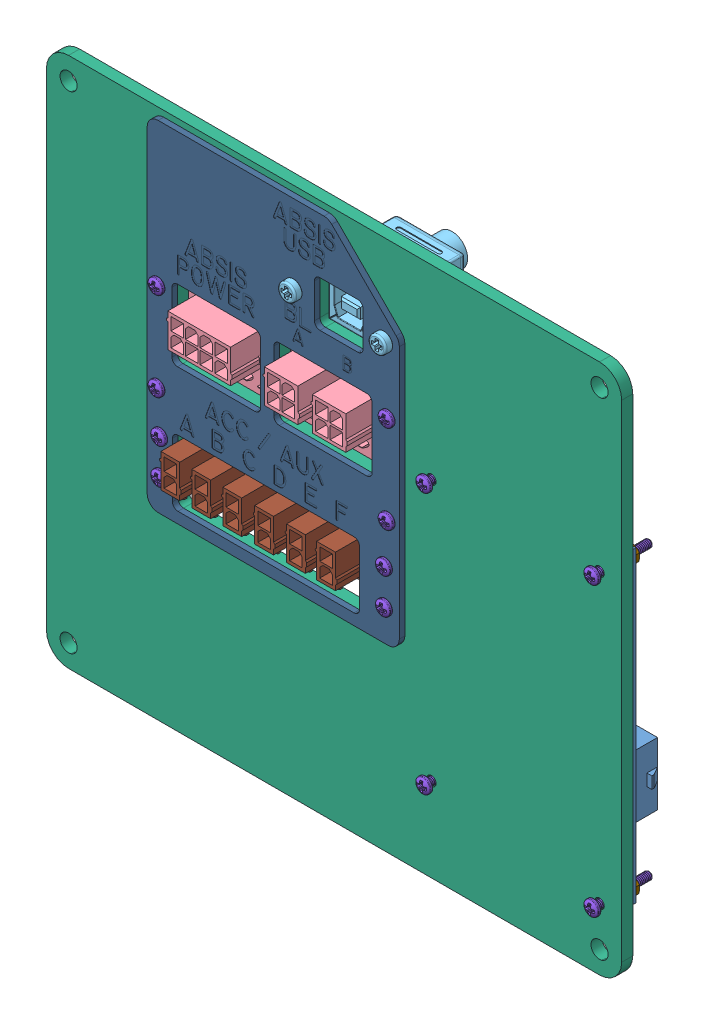
SolidWorks assembly Right Console Bulkhead Interconnect Panel, configuration Default. Lengths in mm.
Overall size (165.1 152.4 37.41).
47 component instances, 11 part files, 24 mates.
Components (placement in the parent):
- ABSIS_hid_bus_master_pcb-1: ABSIS_hid_bus_master_pcb [Default] at (-289.2033 2614.9961 -5883.3904) x (0 -1 0) z (0 0 -1) size (90.8 53.34 16.58)
  - ABSIS_hid_bus_master_pcb-1: ABSIS_hid_bus_master_pcb [Default] at (-243.5501 4.8834 76.9629) size (90.8 53.34 16.58)
  - HEADER, PIN, .1 SPACING-1: HEADER, PIN, .1 SPACING [1x12] at (-216.2801 51.8534 85.1199) x (-1 0 0) z (0 -1 0) size (30.48 11.54 2.54)
  - DEV-12640 - ARDUINO PRO MICRO, 5V, 16 MHz, SPARKFUN-1: DEV-12640 - ARDUINO PRO MICRO, 5V, 16 MHz, SPARKFUN [Default] at (-217.5501 37.8834 85.1199) x (1 0 0) z (0 -1 0) size (34.59 4.25 17.78)
  - HEADER, PIN, .1 SPACING-2: HEADER, PIN, .1 SPACING [1x12] at (-216.2801 36.6134 85.1199) x (-1 0 0) z (0 -1 0) size (30.48 11.54 2.54)
- ABSIS_Bulkhead_Connector-1: ABSIS_Bulkhead_Connector [Default] at (-525.8617 2925.8262 -5961.9533) x (1 0 0) z (0 0 1) size (76.2 35.56 27.3)
- 1581-01C - CABLE, USB 2.0, TYPE B FEMALE TO MICRO B MALE, 1 FT-1: 1581-01C - CABLE, USB 2.0, TYPE B FEMALE TO MICRO B MALE, 1 FT [USB TYPE B FEMALE] at (-369.8767 2883.2962 -6284.3783) x (-1 -0.000084 0) z (0 0 1) size (33.5 14.04 34.59)
- Right Console Bulkhead Connector Panel^OH5A1-1 - ASSY, RIGHT CONSOLE-1: Right Console Bulkhead Connector Panel^OH5A1-1 - ASSY, RIGHT CONSOLE [Default] at (-0.0817 1.6812 -5954.0033) x (-1 0 0) z (0 0 -1) size (165.1 152.4 3.17)
- 1581-01C - CABLE, USB 2.0, TYPE B FEMALE TO MICRO B MALE, 1 FT-2: 1581-01C - CABLE, USB 2.0, TYPE B FEMALE TO MICRO B MALE, 1 FT [USB TYPE B MICRO MALE] at (-334.7067 2858.208 -5971.2853) x (1 0 0) z (0 1 0) size (10.7 7.58 34.44)
- 94639A187 - SPACER, 2 X .250 OD X .125 L, NYL-1: 94639A187 - SPACER, 2 X .250 OD X .125 L, NYL [94639A187] at (-296.6267 2855.3712 -5958.7658) x (0.961477 0.274887 0) z (0 0 1) size (6.35 6.35 3.17)
- 91249A060 - PHS, 2-56 X .625, 18-8, BLACK OXIDE-2: 91249A060 - PHS, 2-56 X .625, 18-8, BLACK OXIDE [91249A060] at (-296.6267 2855.3712 -5968.2908) x (1 0 0) z (0 0 1) size (4.24 4.24 17.48)
- 95130A105 - NUT, 2-56, NARROW, BRASS-1: 95130A105 - NUT, 2-56, NARROW, BRASS [95130A105] at (-296.6267 2855.3712 -5962.747) x (0.996294 -0.086016 0) z (-0.086016 -0.996294 0) size (3.97 1.94 4.58)
- 95130A105 - NUT, 2-56, NARROW, BRASS-2: 95130A105 - NUT, 2-56, NARROW, BRASS [95130A105] at (-355.6817 2839.4662 -5962.747) x (0.996294 -0.086016 0) z (-0.086016 -0.996294 0) size (3.97 1.94 4.58)
- 95130A105 - NUT, 2-56, NARROW, BRASS-3: 95130A105 - NUT, 2-56, NARROW, BRASS [95130A105] at (-421.7217 2839.4662 -5962.747) x (0.996294 -0.086016 0) z (-0.086016 -0.996294 0) size (3.97 1.94 4.58)
- 95130A105 - NUT, 2-56, NARROW, BRASS-4: 95130A105 - NUT, 2-56, NARROW, BRASS [95130A105] at (-355.6817 2864.8662 -5962.747) x (0.996294 -0.086016 0) z (-0.086016 -0.996294 0) size (3.97 1.94 4.58)
- 95130A105 - NUT, 2-56, NARROW, BRASS-5: 95130A105 - NUT, 2-56, NARROW, BRASS [95130A105] at (-421.7217 2864.8662 -5962.747) x (0.996294 -0.086016 0) z (-0.086016 -0.996294 0) size (3.97 1.94 4.58)
- 95130A105 - NUT, 2-56, NARROW, BRASS-6: 95130A105 - NUT, 2-56, NARROW, BRASS [95130A105] at (-344.8867 2779.1712 -5962.747) x (0.996294 -0.086016 0) z (-0.086016 -0.996294 0) size (3.97 1.94 4.58)
- 95130A105 - NUT, 2-56, NARROW, BRASS-7: 95130A105 - NUT, 2-56, NARROW, BRASS [95130A105] at (-296.6267 2772.8212 -5962.747) x (0.996294 -0.086016 0) z (-0.086016 -0.996294 0) size (3.97 1.94 4.58)
- 95130A105 - NUT, 2-56, NARROW, BRASS-8: 95130A105 - NUT, 2-56, NARROW, BRASS [95130A105] at (-344.8867 2854.1012 -5962.747) x (0.996294 -0.086016 0) z (-0.086016 -0.996294 0) size (3.97 1.94 4.58)
- 91249A060 - PHS, 2-56 X .625, 18-8, BLACK OXIDE-3: 91249A060 - PHS, 2-56 X .625, 18-8, BLACK OXIDE [91249A060] at (-355.6817 2839.4662 -5968.2908) x (1 0 0) z (0 0 1) size (4.24 4.24 17.48)
- 91249A060 - PHS, 2-56 X .625, 18-8, BLACK OXIDE-4: 91249A060 - PHS, 2-56 X .625, 18-8, BLACK OXIDE [91249A060] at (-421.7217 2839.4662 -5968.2908) x (1 0 0) z (0 0 1) size (4.24 4.24 17.48)
- 91249A060 - PHS, 2-56 X .625, 18-8, BLACK OXIDE-5: 91249A060 - PHS, 2-56 X .625, 18-8, BLACK OXIDE [91249A060] at (-355.6817 2864.8662 -5968.2908) x (1 0 0) z (0 0 1) size (4.24 4.24 17.48)
- 91249A060 - PHS, 2-56 X .625, 18-8, BLACK OXIDE-6: 91249A060 - PHS, 2-56 X .625, 18-8, BLACK OXIDE [91249A060] at (-421.7217 2864.8662 -5968.2908) x (1 0 0) z (0 0 1) size (4.24 4.24 17.48)
- 91249A060 - PHS, 2-56 X .625, 18-8, BLACK OXIDE-7: 91249A060 - PHS, 2-56 X .625, 18-8, BLACK OXIDE [91249A060] at (-344.8867 2779.1712 -5968.2908) x (1 0 0) z (0 0 1) size (4.24 4.24 17.48)
- 91249A060 - PHS, 2-56 X .625, 18-8, BLACK OXIDE-8: 91249A060 - PHS, 2-56 X .625, 18-8, BLACK OXIDE [91249A060] at (-296.6267 2772.8212 -5968.2908) x (1 0 0) z (0 0 1) size (4.24 4.24 17.48)
- 91249A060 - PHS, 2-56 X .625, 18-8, BLACK OXIDE-9: 91249A060 - PHS, 2-56 X .625, 18-8, BLACK OXIDE [91249A060] at (-344.8867 2854.1012 -5968.2908) x (1 0 0) z (0 0 1) size (4.24 4.24 17.48)
- 94639A187 - SPACER, 2 X .250 OD X .125 L, NYL-2: 94639A187 - SPACER, 2 X .250 OD X .125 L, NYL [94639A187] at (-355.6817 2839.4662 -5958.7658) x (0.961477 0.274887 0) z (0 0 1) size (6.35 6.35 3.17)
- 94639A187 - SPACER, 2 X .250 OD X .125 L, NYL-3: 94639A187 - SPACER, 2 X .250 OD X .125 L, NYL [94639A187] at (-421.7217 2839.4662 -5958.7658) x (0.961477 0.274887 0) z (0 0 1) size (6.35 6.35 3.17)
- 94639A187 - SPACER, 2 X .250 OD X .125 L, NYL-4: 94639A187 - SPACER, 2 X .250 OD X .125 L, NYL [94639A187] at (-355.6817 2864.8662 -5958.7658) x (0.961477 0.274887 0) z (0 0 1) size (6.35 6.35 3.17)
- 94639A187 - SPACER, 2 X .250 OD X .125 L, NYL-5: 94639A187 - SPACER, 2 X .250 OD X .125 L, NYL [94639A187] at (-421.7217 2864.8662 -5958.7658) x (0.961477 0.274887 0) z (0 0 1) size (6.35 6.35 3.17)
- 94639A187 - SPACER, 2 X .250 OD X .125 L, NYL-6: 94639A187 - SPACER, 2 X .250 OD X .125 L, NYL [94639A187] at (-344.8867 2779.1712 -5958.7658) x (0.961477 0.274887 0) z (0 0 1) size (6.35 6.35 3.17)
- 94639A187 - SPACER, 2 X .250 OD X .125 L, NYL-7: 94639A187 - SPACER, 2 X .250 OD X .125 L, NYL [94639A187] at (-296.6267 2772.8212 -5958.7658) x (0.961477 0.274887 0) z (0 0 1) size (6.35 6.35 3.17)
- 94639A187 - SPACER, 2 X .250 OD X .125 L, NYL-8: 94639A187 - SPACER, 2 X .250 OD X .125 L, NYL [94639A187] at (-344.8867 2854.1012 -5958.7658) x (0.961477 0.274887 0) z (0 0 1) size (6.35 6.35 3.17)
- Right Console Bulkhead Interconnect Panel Legend Plate-1: Right Console Bulkhead Interconnect Panel Legend Plate [Default] at (0 0 -5954.0033) x (1 0 0) z (0 0 1) size (72.39 97.5 1.59)
- ABSIS_AUX_Bulkhead_Connector-1: ABSIS_AUX_Bulkhead_Connector [Default] at (-525.0997 2888.6787 -5961.9533) x (1 0 0) z (0 0 1) size (74.68 20.32 27.3)
- 94639A187 - SPACER, 2 X .250 OD X .125 L, NYL-9: 94639A187 - SPACER, 2 X .250 OD X .125 L, NYL [94639A187] at (-356.4437 2817.5587 -5958.7658) x (0.961477 0.274887 0) z (0 0 1) size (6.35 6.35 3.17)
- 94639A187 - SPACER, 2 X .250 OD X .125 L, NYL-10: 94639A187 - SPACER, 2 X .250 OD X .125 L, NYL [94639A187] at (-356.4437 2827.7187 -5958.7658) x (0.961477 0.274887 0) z (0 0 1) size (6.35 6.35 3.17)
- 94639A187 - SPACER, 2 X .250 OD X .125 L, NYL-11: 94639A187 - SPACER, 2 X .250 OD X .125 L, NYL [94639A187] at (-420.9597 2817.5587 -5958.7658) x (0.961477 0.274887 0) z (0 0 1) size (6.35 6.35 3.17)
- 94639A187 - SPACER, 2 X .250 OD X .125 L, NYL-12: 94639A187 - SPACER, 2 X .250 OD X .125 L, NYL [94639A187] at (-420.9597 2827.7187 -5958.7658) x (0.961477 0.274887 0) z (0 0 1) size (6.35 6.35 3.17)
- 91249A060 - PHS, 2-56 X .625, 18-8, BLACK OXIDE-10: 91249A060 - PHS, 2-56 X .625, 18-8, BLACK OXIDE [91249A060] at (-356.4437 2817.5587 -5968.2908) x (1 0 0) z (0 0 1) size (4.24 4.24 17.48)
- 91249A060 - PHS, 2-56 X .625, 18-8, BLACK OXIDE-11: 91249A060 - PHS, 2-56 X .625, 18-8, BLACK OXIDE [91249A060] at (-356.4437 2827.7187 -5968.2908) x (1 0 0) z (0 0 1) size (4.24 4.24 17.48)
- 91249A060 - PHS, 2-56 X .625, 18-8, BLACK OXIDE-12: 91249A060 - PHS, 2-56 X .625, 18-8, BLACK OXIDE [91249A060] at (-420.9597 2817.5587 -5968.2908) x (1 0 0) z (0 0 1) size (4.24 4.24 17.48)
- 91249A060 - PHS, 2-56 X .625, 18-8, BLACK OXIDE-13: 91249A060 - PHS, 2-56 X .625, 18-8, BLACK OXIDE [91249A060] at (-420.9597 2827.7187 -5968.2908) x (1 0 0) z (0 0 1) size (4.24 4.24 17.48)
- 95130A105 - NUT, 2-56, NARROW, BRASS-9: 95130A105 - NUT, 2-56, NARROW, BRASS [95130A105] at (-356.4437 2817.5587 -5962.747) x (0.996294 -0.086016 0) z (-0.086016 -0.996294 0) size (3.97 1.94 4.58)
- 95130A105 - NUT, 2-56, NARROW, BRASS-10: 95130A105 - NUT, 2-56, NARROW, BRASS [95130A105] at (-356.4437 2827.7187 -5962.747) x (0.996294 -0.086016 0) z (-0.086016 -0.996294 0) size (3.97 1.94 4.58)
- 95130A105 - NUT, 2-56, NARROW, BRASS-11: 95130A105 - NUT, 2-56, NARROW, BRASS [95130A105] at (-420.9597 2817.5587 -5962.747) x (0.996294 -0.086016 0) z (-0.086016 -0.996294 0) size (3.97 1.94 4.58)
- 95130A105 - NUT, 2-56, NARROW, BRASS-12: 95130A105 - NUT, 2-56, NARROW, BRASS [95130A105] at (-420.9597 2827.7187 -5962.747) x (0.996294 -0.086016 0) z (-0.086016 -0.996294 0) size (3.97 1.94 4.58)
Mates (geometry in assembly coordinates):
- Distance5: distance = 3.175 mm anti-aligned: plane of ABSIS_hid_bus_master_pcb-1/ABSIS_hid_bus_master_pcb-1 through (-320.5698 2813.9836 -5960.3533) normal (0 0 1); plane of Right Console Bulkhead Connector Panel^OH5A1-1 - ASSY, RIGHT CONSOLE-1 through (-0.0817 1.6812 -5957.1783) normal (0 0 -1)
- Distance6: distance = 6.35 mm: cylinder of ABSIS_hid_bus_master_pcb-1/ABSIS_hid_bus_master_pcb-1 through (-296.6267 2772.8212 -5959.5533) axis (0 0 -1) radius 1.524; plane of Right Console Bulkhead Connector Panel^OH5A1-1 - ASSY, RIGHT CONSOLE-1 through (-290.2767 2907.4412 -5957.1783) normal (1 0 0)
- Distance7: distance = 6.35 mm: plane of ABSIS_hid_bus_master_pcb-1/ABSIS_hid_bus_master_pcb-1 through (-297.8967 2767.7412 -5960.3533) normal (0 -1 0); cylinder of Right Console Bulkhead Connector Panel^OH5A1-1 - ASSY, RIGHT CONSOLE-1 through (-296.6267 2761.3912 -5957.1783) axis (0 0 -1) radius 2.4574
- Parallel19: parallel aligned: plane of ABSIS_hid_bus_master_pcb-1/ABSIS_hid_bus_master_pcb-1 through (-294.0867 2858.5462 -5960.3533) normal (1 0 0); plane of Right Console Bulkhead Connector Panel^OH5A1-1 - ASSY, RIGHT CONSOLE-1 through (-290.2767 2907.4412 -5957.1783) normal (1 0 0)
- Distance8: distance = 12.7 mm anti-aligned: plane of 1581-01C - CABLE, USB 2.0, TYPE B FEMALE TO MICRO B MALE, 1 FT-1 through (-360.1267 2876.2962 -5979.5783) normal (1 0 0); plane of ABSIS_hid_bus_master_pcb-1/ABSIS_hid_bus_master_pcb-1 through (-347.4267 2772.8212 -5960.3533) normal (-1 0 0)
- Parallel20: parallel aligned: plane of ABSIS_hid_bus_master_pcb-1/DEV-12640 - ARDUINO PRO MICRO, 5V, 16 MHz, SPARKFUN-1 through (-331.4567 2832.2962 -5972.4603) normal (0 0 -1); plane of 1581-01C - CABLE, USB 2.0, TYPE B FEMALE TO MICRO B MALE, 1 FT-2 through (-337.6867 2849.666 -5972.1703) normal (0 0 -1)
- Symmetric1: symmetric aligned: plane of ABSIS_hid_bus_master_pcb-1/DEV-12640 - ARDUINO PRO MICRO, 5V, 16 MHz, SPARKFUN-1 through (-338.4067 2832.2962 -5972.0103) normal (-1 0 0); plane of 1581-01C - CABLE, USB 2.0, TYPE B FEMALE TO MICRO B MALE, 1 FT-2 through (-331.0067 2832.2962 -5971.1931) normal (1 0 0); plane of ABSIS_hid_bus_master_pcb-1/DEV-12640 - ARDUINO PRO MICRO, 5V, 16 MHz, SPARKFUN-1 through (-334.7067 2858.208 -5971.2853) normal (1 0 0)
- Symmetric2: symmetric aligned: plane of ABSIS_hid_bus_master_pcb-1/DEV-12640 - ARDUINO PRO MICRO, 5V, 16 MHz, SPARKFUN-1 through (-331.4567 2832.2962 -5972.4603) normal (0 0 -1); plane of 1581-01C - CABLE, USB 2.0, TYPE B FEMALE TO MICRO B MALE, 1 FT-2 through (-334.7067 2832.2962 -5970.1103) normal (0 0 1); plane of ABSIS_hid_bus_master_pcb-1/DEV-12640 - ARDUINO PRO MICRO, 5V, 16 MHz, SPARKFUN-1 through (-334.7067 2858.208 -5971.2853) normal (0 0 -1)
- Coincident197: coincident: line of ABSIS_hid_bus_master_pcb-1/DEV-12640 - ARDUINO PRO MICRO, 5V, 16 MHz, SPARKFUN-1 through (-331.9317 2836.2962 -5972.6274) axis (-1 0 0); plane of 1581-01C - CABLE, USB 2.0, TYPE B FEMALE TO MICRO B MALE, 1 FT-2 through (-332.1317 2836.2962 -5972.6753) normal (0 1 0)
- Distance9: distance = 9.525 mm anti-aligned: plane of ABSIS_Bulkhead_Connector-1 through (-387.9565 2818.735 -5967.73) normal (0 0 1); plane of Right Console Bulkhead Connector Panel^OH5A1-1 - ASSY, RIGHT CONSOLE-1 through (0 0 -5958.205) normal (0 0 -1)
- Distance10: distance = 6.35 mm anti-aligned: plane of ABSIS_Bulkhead_Connector-1 through (-426.8017 2869.9462 -5961.9533) normal (0 1 0); plane of 1581-01C - CABLE, USB 2.0, TYPE B FEMALE TO MICRO B MALE, 1 FT-1 through (-379.6267 2876.2962 -5979.5783) normal (0 -1 0)
- Coincident195: coincident anti-aligned: plane of Right Console Bulkhead Connector Panel^OH5A1-1 - ASSY, RIGHT CONSOLE-1 through (-0.0817 1.6812 -5957.1783) normal (0 0 -1); plane of 1581-01C - CABLE, USB 2.0, TYPE B FEMALE TO MICRO B MALE, 1 FT-1 through (-369.8767 2883.2962 -5957.1783) normal (0 0 1)
- Distance11: distance = 3.175 mm anti-aligned: plane of ABSIS_Bulkhead_Connector-1 through (-388.7017 2852.1662 -5960.3533) normal (0 0 1); plane of Right Console Bulkhead Connector Panel^OH5A1-1 - ASSY, RIGHT CONSOLE-1 through (-0.0817 1.6812 -5957.1783) normal (0 0 -1)
- Distance12: distance = 3.175 mm anti-aligned: plane of ABSIS_hid_bus_master_pcb-1/ABSIS_hid_bus_master_pcb-1 through (-347.4267 2772.8212 -5960.3533) normal (-1 0 0); plane of ABSIS_Bulkhead_Connector-1 through (-350.6017 2869.9462 -5961.9533) normal (1 0 0)
- Concentric1: concentric aligned: cylinder of Right Console Bulkhead Connector Panel^OH5A1-1 - ASSY, RIGHT CONSOLE-1 through (-296.6267 2855.3712 -5957.1783) axis (0 0 -1) radius 1.3526; cylinder of 94639A187 - SPACER, 2 X .250 OD X .125 L, NYL-1 through (-296.6267 2855.3712 -5957.1783) axis (0 0 -1) radius 3.175
- Coincident198: coincident anti-aligned: plane of Right Console Bulkhead Connector Panel^OH5A1-1 - ASSY, RIGHT CONSOLE-1 through (-0.0817 1.6812 -5957.1783) normal (0 0 -1); plane of 94639A187 - SPACER, 2 X .250 OD X .125 L, NYL-1 through (-296.6267 2855.3712 -5957.1783) normal (0 0 1)
- Concentric3: concentric aligned: cylinder of Right Console Bulkhead Connector Panel^OH5A1-1 - ASSY, RIGHT CONSOLE-1 through (-296.6267 2855.3712 -5957.1783) axis (0 0 -1) radius 1.3526; cylinder of 91249A060 - PHS, 2-56 X .625, 18-8, BLACK OXIDE-2 through (-296.6267 2855.3712 -5968.2908) axis (0 0 -1) radius 2.1209
- Concentric4: concentric anti-aligned: circle of ABSIS_hid_bus_master_pcb-1/ABSIS_hid_bus_master_pcb-1; circle of 95130A105 - NUT, 2-56, NARROW, BRASS-1
- Coincident200: coincident anti-aligned: plane of ABSIS_hid_bus_master_pcb-1/ABSIS_hid_bus_master_pcb-1 through (-320.5698 2813.9836 -5961.9533) normal (0 0 -1); plane of 95130A105 - NUT, 2-56, NARROW, BRASS-1 through (-298.5052 2856.6834 -5961.9533) normal (0 0 1)
- Distance13: distance = 1.5875 mm anti-aligned: plane of 91249A060 - PHS, 2-56 X .625, 18-8, BLACK OXIDE-2 through (-296.6267 2855.3712 -5952.4158) normal (0 0 -1); plane of Right Console Bulkhead Connector Panel^OH5A1-1 - ASSY, RIGHT CONSOLE-1 through (-0.0817 1.6812 -5954.0033) normal (0 0 1)
- Coincident204: coincident aligned: plane of ABSIS_Bulkhead_Connector-1 through (-388.7017 2852.1662 -5961.9533) normal (0 0 -1); plane of ABSIS_AUX_Bulkhead_Connector-1 through (-388.7017 2822.6387 -5961.9533) normal (0 0 -1)
- Distance16: distance = 1.5875 mm anti-aligned: plane of ABSIS_AUX_Bulkhead_Connector-1 through (-426.0397 2832.7987 -5961.9533) normal (0 1 0); plane of ABSIS_Bulkhead_Connector-1 through (-350.6017 2834.3862 -5961.9533) normal (0 -1 0)
- Width1: width anti-aligned: plane of ABSIS_Bulkhead_Connector-1 through (-350.6017 2869.9462 -5961.9533) normal (1 0 0); plane of ABSIS_AUX_Bulkhead_Connector-1 through (-426.8017 2834.3862 -5961.9533) normal (-1 0 0); plane of ABSIS_Bulkhead_Connector-1 through (-426.0397 2812.4787 -5961.9533) normal (-1 0 0); plane of ABSIS_AUX_Bulkhead_Connector-1 through (-351.3637 2832.7987 -5961.9533) normal (1 0 0)
- Distance17: distance = 31.75 mm aligned: plane of 1581-01C - CABLE, USB 2.0, TYPE B FEMALE TO MICRO B MALE, 1 FT-1 through (-360.1267 2890.2962 -5979.5783) normal (0 1 0); plane of ABSIS_hid_bus_master_pcb-1/ABSIS_hid_bus_master_pcb-1 through (-347.4267 2858.5462 -5960.3533) normal (0 1 0)
